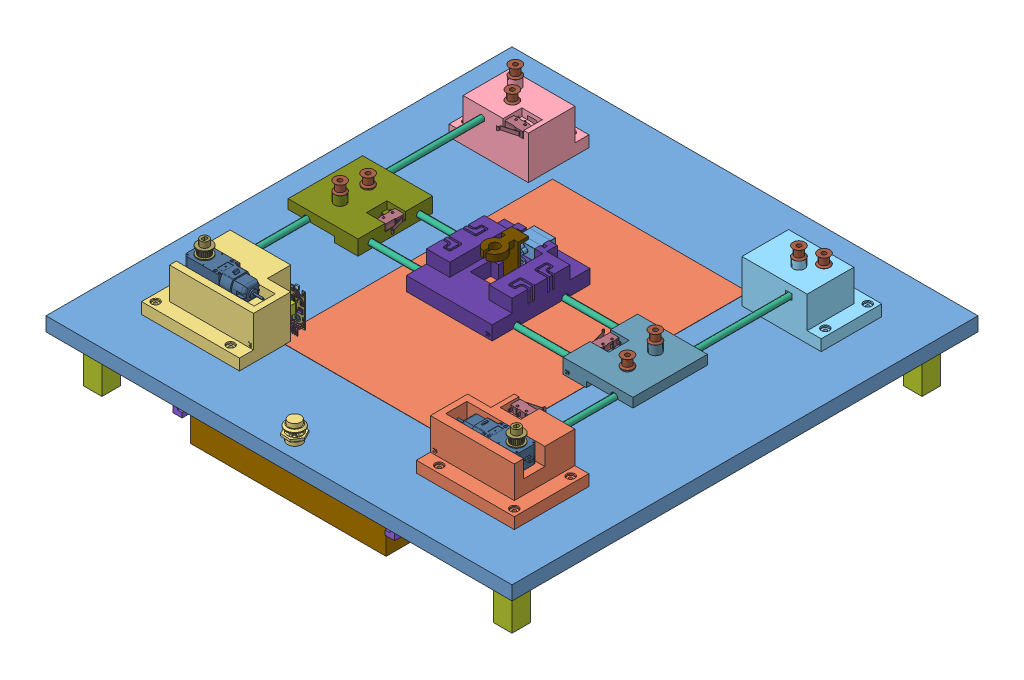
SolidWorks assembly Assem1.1, configuration Default. Lengths in mm.
Overall size (500 139.59 500).
80 component instances, 49 part files, 171 mates.
Components (placement in the parent):
- Base-1: Base [Default] at (441.6833 230.1614 146.9363) size (500 15 500)
- STEPPER RIGHT-1: STEPPER RIGHT [Default] at (291.6086 245.1614 514.4363) size (105 46 80)
- STEPPER LEFT-1: STEPPER LEFT [Default] at (91.7583 245.1614 579.4363) x (0 0 1) z (0 1 0) size (80 105 46)
- TOP RIGHT-1: TOP RIGHT [Default] at (6.7583 245.1614 214.4363) size (85 56 65)
- TOP LEFT-1: TOP LEFT [Default] at (377.872 245.1614 264.4363) x (0 0 1) z (-1 0 0) size (65 54.7 85)
- Shaft-2: Shaft [Default] at (26.7583 280.1614 234.4363) x (0.670425 0.741977 0) z (0.741977 -0.670425 0) size (6 300 6)
- FOOT-1: FOOT [Default] at (-38.3167 180.1614 606.9363) size (40 50 40)
- FOOT-2: FOOT [Default] at (401.6833 180.1614 606.9363) size (40 50 40)
- FOOT-3: FOOT [Default] at (401.6833 180.1614 166.9363) size (40 50 40)
- FOOT-4: FOOT [Default] at (-38.3167 180.1614 166.9363) size (40 50 40)
- STORAGE SUPPORT-1: STORAGE SUPPORT [Default] at (318.6833 225.1614 481.9363) x (-1 0 0) z (0 1 0) size (18 160 12)
- STORAGE SUPPORT-2: STORAGE SUPPORT [Default] at (64.6833 225.1614 641.9363) x (1 0 0) z (0 1 0) size (18 160 12)
- STORAGE-2: STORAGE [Default] at (91.6833 199.1614 632.0504) x (1 0 0) z (0 0 -1) size (226 35 155)
- DG01D Motor-1: DG01D Motor [Default] at (25.7583 300.9614 560.8363) x (-1 0 0) z (0 1 0) size (79.2 22.5 37.6)
- DG01D Motor-2: DG01D Motor [Default] at (357.6086 291.1614 558.0363) x (1 0 0) z (0 1 0) size (79.2 22.5 37.6)
- Pully-3: Pully [Default] at (345.0586 304.8614 242.4363) x (-1 0 0) z (0 0 1) size (12.7 10 12.7)
- Pully-4: Pully [Default] at (356.9086 296.1614 227.4363) x (-1 0 0) z (0 0 1) size (12.7 10 12.7)
- GT2 20T motor-1: GT2 20T motor [Default] at (25.7583 309.4614 560.8363) x (1 0 0) z (0 1 0) size (16 16 15)
- GT2 20T motor-2: GT2 20T motor [Default] at (357.6086 299.6614 558.0363) x (1 0 0) z (0 1 0) size (16 16 15)
- Pully-9: Pully [Default] at (25.7583 306.1614 227.4363) x (-1 0 0) z (0 0 1) size (12.7 10 12.7)
- Pully-10: Pully [Default] at (37.6083 296.1614 242.4363) x (-1 0 0) z (0 0 1) size (12.7 10 12.7)
- SS_5GL13.step-3: SS_5GL13.step [Default] at (332.3586 286.3614 522.1363) x (1 0 0) z (0 1 0) size (21.03 22.89 6.4)
- SS_5GL13.step-4: SS_5GL13.step [Default] at (56.0083 286.3614 256.7363) x (-1 0 0) z (0 1 0) size (21.03 22.89 6.4)
- Shaft-8: Shaft [Default] at (356.7586 280.0114 234.4363) x (-0.419242 0.907875 0) z (0.907875 0.419242 0) size (6 300 6)
- END EFFECTOR RIGHT-3: END EFFECTOR RIGHT [Default] at (316.7592 279.469 452.2484) x (0 0 -1) z (0.999999 0.001061 0) size (80 26 75)
- LMU-N6-8: LMU-N6 [Default] at (356.7586 280.0114 411.9984) x (-0.078757 0.996894 0) z (0.996894 0.078757 0) size (12 19 12)
- LMU-N6-9: LMU-N6 [Default] at (26.7583 280.1614 411.9984) x (1 0 0) z (0 1 0) size (12 19 12)
- END EFFECTOR LEFT-3: END EFFECTOR LEFT [Default] at (66.7593 279.2038 372.2484) x (0 0 1) z (-0.999999 -0.001061 0) size (80 26 75)
- Shaft-9: Shaft [Default] at (341.7591 279.4955 438.2484) x (-0.000465 0.43872 0.898624) z (0.000953 -0.898623 0.43872) size (6 300 6)
- Shaft-10: Shaft [Default] at (341.7591 279.4955 386.2484) x (-0.001061 0.999999 0) z (0 0 1) size (6 300 6)
- END EFFECTOR BASE-3: END EFFECTOR BASE [Default] at (238.2479 278.8857 464.7484) x (0 0 -1) z (0.999999 0.001061 0) size (105 29 92)
- LMU-N6-10: LMU-N6 [Default] at (168.7474 279.312 386.2484) x (0.001061 -0.999999 0) z (0 0 1) size (12 19 12)
- LMU-N6-11: LMU-N6 [Default] at (191.7474 279.3364 438.2484) x (0.001043 -0.983378 -0.181565) z (0.000193 -0.181565 0.983379) size (12 19 12)
- LMU-N6-12: LMU-N6 [Default] at (215.7474 279.3618 386.2484) x (0.001061 -0.999999 0) z (0 0 1) size (12 19 12)
- PEN HOLDER NEW-2: PEN HOLDER NEW [Default] at (192.212 312.7416 415.8858) x (0.999999 0.001061 0) z (0 0 1) size (22 52.5 38.03)
- SS_5GL13.step-5: SS_5GL13.step [Default] at (309.4536 284.6612 407.4984) x (0 0 -1) z (-0.001061 0.999999 0) size (21.03 22.89 6.4)
- SS_5GL13.step-6: SS_5GL13.step [Default] at (74.0538 284.4116 416.9984) x (0 0 1) z (-0.001061 0.999999 0) size (21.03 22.89 6.4)
- Pully-11: Pully [Default] at (345.8915 296.0999 427.2484) x (-0.999999 -0.001061 0) z (0 0 1) size (12.7 10 12.7)
- Pully-12: Pully [Default] at (345.8826 304.4999 397.2484) x (-0.999999 -0.001061 0) z (0 0 1) size (12.7 10 12.7)
- Pully-13: Pully [Default] at (37.5828 304.1729 427.2484) x (0.837232 0.000888 0.546848) z (0.546847 0.00058 -0.837232) size (12.7 10 12.7)
- Pully-14: Pully [Default] at (37.5917 295.7729 397.2484) x (-0.999999 -0.001061 0) z (0 0 1) size (12.7 10 12.7)
- servo-1: servo [Default] at (184.3266 318.5665 361.0815) x (0.999999 0.001061 0) z (0.001061 -0.999999 0) size (38.73 33.09 12.1)
- A4_paper-1: A4_paper [Default] at (191.6833 245.1614 396.9363) size (210 0.3 297)
- PushButtonRed-1: PushButtonRed [Default] at (191.0864 258.4614 629.4531) x (-0.837169 0 -0.546944) z (0 1 0) size (19.62 21.94 25.6)
- KY-024 Linear Magnetic Hall Effect Switches.step-3: KY-024 Linear Magnetic Hall Effect Switches.step [Default] at (93.976 267.3857 527.7213) x (0 1 0) z (1 0 0) size (43.63 13.45 15)
  - Sensor.step-1: Sensor.step [Default] at (21.0875 1.0886 -0.8799) x (0 0 -1) z (0 -1 0) size (6.43 12.72 3.32)
    - Pins.step-1: Pins.step [Default] at origin size (5.99 9.68 3.16)
    - Sensor-0.step-1: Sensor-0.step [Default] at origin size (4.1 3.2 1.5)
  - Fusion002.step-1: Fusion002.step [Default] at (2.0698 -0.285 -0.8494) x (0 0 1) z (0 1 0) size (14.06 29.56 0.01)
  - Trimpot.step-1: Trimpot.step [Default] at (0.8941 5.715 -1.9169) x (0 1 0) z (1 0 0) size (13.19 5 10)
  - lm393.step-1: lm393.step [Default] at (16.3888 -1.3356 -7.4144) x (-1 0 0) z (0 1 0) size (4.98 4.98 1.83)
  - Pad003.step-1: Pad003.step [Default] at (2.0698 0.725 -0.8494) x (0 0 1) z (0 1 0) size (14.68 24.36 0.01)
  - Pad001.step-1: Pad001.step [Default] at (2.0698 -0.294 -0.8494) x (0 0 1) z (0 1 0) size (13.63 28.59 1.03)
  - Pad002.step-1: Pad002.step [Default] at (2.0698 0.725 -0.8494) x (0 0 1) z (0 1 0) size (9.53 3.34 0.01)
  - PCB.step-1: PCB.step [Default] at (2.0698 -0.285 -0.8494) x (0 0 1) z (0 1 0) size (15 35 1)
  - PIN HEADER, 1X4, 2.54 mm.step-1: PIN HEADER, 1X4, 2.54 mm.step [Default] at (-13.6966 0.693 -2.0725) x (0 0 -1) z (1 0 0) size (10.08 6.81 8.5)
  - Led.step-1: Led.step [Default] at (0.9398 -1.2392 1.8074) x (-1 0 0) z (0 1 0) size (2.66 1.33 0.62)
  - Led (1).step-1: Led (1).step [Default] at (2.913 -0.8113 -18.8497) size (2.66 0.62 1.33)
  - Resistor.step-1: Resistor.step [Default] at origin size (2.57 0.86 1.53)
  - Resistor (1).step-1: Resistor (1).step [Default] at (0 0 -2.456) size (2.57 0.86 1.53)
  - Resistor (2).step-1: Resistor (2).step [Default] at (0 0 -9.9569) size (2.57 0.86 1.53)
  - Resistor (3).step-1: Resistor (3).step [Default] at (0 0 -12.4652) size (2.57 0.86 1.53)
  - Resistor (4).step-1: Resistor (4).step [Default] at (-18.4143 0 0.076) size (2.57 0.86 1.53)
  - Resistor (5).step-1: Resistor (5).step [Default] at (-18.5044 0 -12.6045) size (2.57 0.86 1.53)
  - Pad (2).step-1: Pad (2).step [Default] at origin size (1.8 0.7 1.8)
  - Pad (4).step-1: Pad (4).step [Default] at origin size (1.8 0.7 1.8)
  - Pad (3).step-1: Pad (3).step [Default] at origin size (1.8 0.7 1.8)
  - Pad (5).step-1: Pad (5).step [Default] at origin size (1.8 0.7 1.8)
  - Pad (2) (1).step-1: Pad (2) (1).step [Default] at (12.1225 0 -7.5843) size (1.8 0.7 1.8)
  - Pad (2) (2).step-1: Pad (2) (2).step [Default] at (14.6713 0 -7.6465) size (1.8 0.7 1.8)
  - Pad (2) (3).step-1: Pad (2) (3).step [Default] at (17.0958 0 -7.5843) size (1.8 0.7 1.8)
  - Pad.step-1: Pad.step [Default] at origin size (1.6 1.01 1.6)
  - Pad (1).step-1: Pad (1).step [Default] at origin size (1.6 1.01 1.6)
  - Pad (6).step-1: Pad (6).step [Default] at origin size (1.6 1.01 1.6)
  - Pad (2) (3).step-2: Pad (2) (3).step [Default] at (23.9554 0.5875 6.0878) x (1 0 0) z (0 0 -1) size (1.8 0.7 1.8)
  - Pad (2) (3).step-3: Pad (2) (3).step [Default] at (25.2062 0.5875 3.4651) x (1 0 0) z (0 0 -1) size (1.8 0.7 1.8)
  - Pad (2) (3).step-4: Pad (2) (3).step [Default] at (25.2466 0.5875 0.8827) x (1 0 0) z (0 0 -1) size (1.8 0.7 1.8)
  - Pad (2) (3).step-5: Pad (2) (3).step [Default] at (25.2466 -0.0666 -4.9814) size (1.8 0.7 1.8)
  - Pad (2) (3).step-6: Pad (2) (3).step [Default] at (25.2466 -0.0666 -2.5658) size (1.8 0.7 1.8)
  - Pad (2) (3).step-7: Pad (2) (3).step [Default] at (23.8777 -0.0666 0.2122) size (1.8 0.7 1.8)
Mates (geometry in assembly coordinates):
- Coincident1: coincident anti-aligned: plane of Base-1 through (441.6833 245.1614 146.9363) normal (0 1 0); plane of STEPPER RIGHT-1 through (291.6086 245.1614 514.4363) normal (0 -1 0)
- Coincident2: coincident anti-aligned: plane of Base-1 through (441.6833 245.1614 146.9363) normal (0 1 0); plane of STEPPER LEFT-1 through (91.7583 245.1614 579.4363) normal (0 -1 0)
- Coincident3: coincident anti-aligned: plane of Base-1 through (441.6833 245.1614 146.9363) normal (0 1 0); plane of TOP RIGHT-1 through (6.7583 245.1614 214.4363) normal (0 -1 0)
- Coincident4: coincident anti-aligned: plane of Base-1 through (441.6833 245.1614 146.9363) normal (0 1 0); plane of TOP LEFT-1 through (377.872 245.1614 264.4363) normal (0 -1 0)
- Tangent12: tangent anti-aligned: plane of TOP LEFT-1 through (352.7586 277.0114 234.4363) normal (0 1 0); cylinder of Shaft-3 through (357.1083 280.0114 529.4363) axis (0 0 -1) radius 3
- Concentric3: concentric anti-aligned: cylinder of Shaft-3 through (357.1083 280.0114 529.4363) axis (0 0 -1) radius 3; cylinder of LMU-N6-1 through (376.7583 280.0114 378.9727) axis (0 0 1) radius 3
- Concentric4: concentric aligned: cylinder of END EFFECTOR LEFT-1 through (376.7583 280.0114 378.4727) axis (0 0 1) radius 6; cylinder of LMU-N6-1 through (376.7583 280.0114 378.9727) axis (0 0 1) radius 6
- Coincident13: coincident anti-aligned: plane of END EFFECTOR LEFT-1 through (376.7583 280.0114 397.9727) normal (0 0 -1); plane of LMU-N6-1 through (376.7583 280.0114 397.9727) normal (0 0 1)
- Concentric5: concentric aligned: cylinder of Shaft-2 through (26.7583 280.1614 534.4363) axis (0 0 -1) radius 3; cylinder of LMU-N6-2 through (46.7579 280.1614 397.4727) axis (0 0 -1) radius 3
- Concentric6: concentric aligned: cylinder of END EFFECTOR RIGHT-1 through (46.7579 280.1614 397.9727) axis (0 0 -1) radius 6; cylinder of LMU-N6-2 through (46.7579 280.1614 397.4727) axis (0 0 -1) radius 6
- Coincident14: coincident anti-aligned: plane of END EFFECTOR RIGHT-1 through (46.7579 280.1614 378.4727) normal (0 0 1); plane of LMU-N6-2 through (46.7579 280.1614 378.4727) normal (0 0 -1)
- Concentric7: concentric anti-aligned: cylinder of END EFFECTOR LEFT-1 through (361.7563 279.0409 414.2227) axis (-0.999998 0.00197 0) radius 3.15; cylinder of Shaft-4 through (61.7569 279.6319 414.2227) axis (0.999998 -0.00197 0) radius 3
- Coincident15: coincident anti-aligned: plane of END EFFECTOR LEFT-1 through (361.7563 279.0409 414.2227) normal (-0.999998 0.00197 0); plane of Shaft-4 through (361.7563 279.0409 414.2227) normal (0.999998 -0.00197 0)
- Concentric8: concentric anti-aligned: cylinder of END EFFECTOR LEFT-1 through (361.7563 279.0409 362.2227) axis (-0.999998 0.00197 0) radius 3.15; cylinder of Shaft-5 through (61.7569 279.6319 362.2227) axis (0.999998 -0.00197 0) radius 3
- Coincident16: coincident anti-aligned: plane of END EFFECTOR LEFT-1 through (361.7563 279.0409 362.2227) normal (-0.999998 0.00197 0); plane of Shaft-5 through (361.7563 279.0409 362.2227) normal (0.999998 -0.00197 0)
- Coincident17: coincident anti-aligned: plane of END EFFECTOR RIGHT-1 through (61.7569 279.6319 414.2227) normal (0.999998 -0.00197 0); plane of Shaft-4 through (61.7569 279.6319 414.2227) normal (-0.999998 0.00197 0)
- Coincident18: coincident anti-aligned: plane of END EFFECTOR RIGHT-1 through (61.7569 279.6319 362.2227) normal (0.999998 -0.00197 0); plane of Shaft-5 through (61.7569 279.6319 362.2227) normal (-0.999998 0.00197 0)
- Concentric9: concentric aligned: cylinder of END EFFECTOR RIGHT-1 through (61.7569 279.6319 362.2227) axis (0.999998 -0.00197 0) radius 3.15; cylinder of Shaft-5 through (61.7569 279.6319 362.2227) axis (0.999998 -0.00197 0) radius 3
- Concentric10: concentric anti-aligned: cylinder of Shaft-5 through (61.7569 279.6319 362.2227) axis (0.999998 -0.00197 0) radius 3; cylinder of LMU-N6-3 through (251.3995 279.2583 362.2227) axis (-0.999998 0.00197 0) radius 3
- Concentric11: concentric aligned: cylinder of Shaft-5 through (61.7569 279.6319 362.2227) axis (0.999998 -0.00197 0) radius 3; cylinder of LMU-N6-4 through (187.3997 279.3844 362.2227) axis (0.999998 -0.00197 0) radius 3
- Concentric12: concentric anti-aligned: cylinder of Shaft-4 through (61.7569 279.6319 414.2227) axis (0.999998 -0.00197 0) radius 3; circle of LMU-N6-5
- Concentric13: concentric aligned: cylinder of END EFFECTOR BASE-2 through (229.3996 279.3017 414.2227) axis (-0.999998 0.00197 0) radius 6; cylinder of LMU-N6-5 through (228.3996 279.3036 414.2227) axis (-0.999998 0.00197 0) radius 6
- Coincident19: coincident anti-aligned: plane of END EFFECTOR BASE-2 through (209.3996 279.341 414.2227) normal (0.999998 -0.00197 0); plane of LMU-N6-5 through (209.3996 279.341 414.2227) normal (-0.999998 0.00197 0)
- Concentric14: concentric aligned: cylinder of END EFFECTOR BASE-2 through (252.3995 279.2563 362.2227) axis (-0.999998 0.00197 0) radius 6; cylinder of LMU-N6-3 through (251.3995 279.2583 362.2227) axis (-0.999998 0.00197 0) radius 6
- Concentric15: concentric aligned: cylinder of END EFFECTOR BASE-2 through (186.3997 279.3863 362.2227) axis (0.999998 -0.00197 0) radius 6; cylinder of LMU-N6-4 through (187.3997 279.3844 362.2227) axis (0.999998 -0.00197 0) radius 6
- Coincident20: coincident anti-aligned: plane of END EFFECTOR BASE-2 through (206.3996 279.347 362.2227) normal (-0.999998 0.00197 0); plane of LMU-N6-4 through (206.3996 279.347 362.2227) normal (0.999998 -0.00197 0)
- Coincident21: coincident anti-aligned: plane of END EFFECTOR BASE-2 through (232.3996 279.2957 362.2227) normal (0.999998 -0.00197 0); plane of LMU-N6-3 through (232.3996 279.2957 362.2227) normal (-0.999998 0.00197 0)
- Coincident22: coincident: plane of END EFFECTOR BASE-2 through (265.4281 293.7307 440.7227) normal (0.00197 0.999998 0); plane of END EFFECTOR TOP-1 through (212.6755 294.0223 310.2117) normal (-0.000676 -1 0)
- Coincident23: coincident anti-aligned: plane of END EFFECTOR BASE-2 through (234.2863 221.7919 373.2227) normal (0 0 1); plane of PEN HOLDER NEW-1 through (219.4672 313.617 373.2227) normal (0 0 -1)
- Distance7: distance = 1 mm anti-aligned: plane of PEN HOLDER NEW-1 through (228.4671 313.5993 373.2227) normal (0.999998 -0.00197 0); plane of END EFFECTOR BASE-2 through (229.3986 278.8017 373.2227) normal (-0.999998 0.00197 0)
- Coincident26: coincident anti-aligned: plane of Base-1 through (441.6833 230.1614 146.9363) normal (0 -1 0); plane of FOOT-1 through (-38.3167 230.1614 606.9363) normal (0 1 0)
- Distance10: distance = 10 mm aligned: plane of Base-1 through (-58.3167 245.1614 146.9363) normal (-1 0 0); plane of FOOT-1 through (-48.3167 225.1614 596.9363) normal (-1 0 0)
- Distance11: distance = 10 mm aligned: plane of FOOT-1 through (-48.3167 225.1614 636.9363) normal (0 0 1); plane of Base-1 through (441.6833 245.1614 646.9363) normal (0 0 1)
- Coincident28: coincident anti-aligned: plane of Base-1 through (441.6833 230.1614 146.9363) normal (0 -1 0); plane of FOOT-2 through (401.6833 230.1614 606.9363) normal (0 1 0)
- Distance13: distance = 10 mm aligned: plane of FOOT-2 through (391.6833 225.1614 636.9363) normal (0 0 1); plane of Base-1 through (441.6833 245.1614 646.9363) normal (0 0 1)
- Distance14: distance = 10 mm aligned: plane of FOOT-2 through (431.6833 225.1614 596.9363) normal (1 0 0); plane of Base-1 through (441.6833 245.1614 146.9363) normal (1 0 0)
- Coincident31: coincident anti-aligned: plane of Base-1 through (441.6833 230.1614 146.9363) normal (0 -1 0); plane of FOOT-3 through (401.6833 230.1614 166.9363) normal (0 1 0)
- Distance15: distance = 10 mm aligned: plane of FOOT-3 through (431.6833 225.1614 156.9363) normal (1 0 0); plane of Base-1 through (441.6833 245.1614 146.9363) normal (1 0 0)
- Distance16: distance = 10 mm aligned: plane of FOOT-3 through (391.6833 225.1614 156.9363) normal (0 0 -1); plane of Base-1 through (441.6833 245.1614 146.9363) normal (0 0 -1)
- Coincident34: coincident anti-aligned: plane of Base-1 through (441.6833 230.1614 146.9363) normal (0 -1 0); plane of FOOT-4 through (-38.3167 230.1614 166.9363) normal (0 1 0)
- Distance17: distance = 10 mm aligned: plane of FOOT-4 through (-48.3167 225.1614 156.9363) normal (0 0 -1); plane of Base-1 through (441.6833 245.1614 146.9363) normal (0 0 -1)
- Distance18: distance = 10 mm aligned: plane of FOOT-4 through (-48.3167 225.1614 156.9363) normal (-1 0 0); plane of Base-1 through (-58.3167 245.1614 146.9363) normal (-1 0 0)
- Coincident37: coincident anti-aligned: plane of Base-1 through (441.6833 230.1614 146.9363) normal (0 -1 0); plane of STORAGE SUPPORT-1 through (310.6833 230.1614 641.9363) normal (0 1 0)
- Coincident38: coincident anti-aligned: plane of Base-1 through (441.6833 230.1614 146.9363) normal (0 -1 0); plane of STORAGE SUPPORT-2 through (72.6833 230.1614 481.9363) normal (0 1 0)
- Distance19: distance = 1 mm anti-aligned: plane of STORAGE-2 through (91.6833 229.1614 632.0504) normal (0 1 0); plane of Base-1 through (441.6833 230.1614 146.9363) normal (0 -1 0)
- Distance20: distance = 137 mm aligned: plane of STORAGE-2 through (304.6833 199.1614 632.0504) normal (1 0 0); plane of Base-1 through (441.6833 245.1614 146.9363) normal (1 0 0)
- Distance22: distance = 1 mm anti-aligned: plane of STORAGE-2 through (304.6833 199.1614 632.0504) normal (1 0 0); plane of STORAGE SUPPORT-1 through (305.6833 230.1614 641.9363) normal (-1 0 0)
- Distance23: distance = 1 mm anti-aligned: plane of STORAGE SUPPORT-2 through (77.6833 230.1614 481.9363) normal (1 0 0); plane of STORAGE-2 through (78.6833 199.1614 632.0504) normal (-1 0 0)
- Distance24: distance = 5 mm aligned: plane of STORAGE SUPPORT-1 through (318.6833 225.1614 641.9363) normal (0 0 1); plane of Base-1 through (441.6833 245.1614 646.9363) normal (0 0 1)
- Distance25: distance = 5 mm aligned: plane of STORAGE SUPPORT-2 through (64.6833 225.1614 641.9363) normal (0 0 1); plane of Base-1 through (441.6833 245.1614 646.9363) normal (0 0 1)
- Concentric16: concentric anti-aligned: cylinder of STEPPER LEFT-1 through (25.7583 228.7114 560.8363) axis (0 1 0) radius 3.25; cylinder of DG01D Motor-1 through (25.7583 291.5645 560.8363) axis (0 -1 0) radius 2.6
- Concentric17: concentric aligned: cylinder of STEPPER LEFT-1 through (38.0583 228.7114 560.8363) axis (0 1 0) radius 2.35; cylinder of DG01D Motor-1 through (38.0583 281.4193 560.8363) axis (0 1 0) radius 1.9
- Coincident39: coincident anti-aligned: plane of STEPPER LEFT-1 through (91.7583 282.1614 579.4363) normal (0 1 0); plane of DG01D Motor-1 through (32.8456 282.1614 559.8363) normal (0 -1 0)
- Concentric18: concentric anti-aligned: cylinder of STEPPER RIGHT-1 through (357.6086 245.3614 558.0363) axis (0 1 0) radius 3.25; cylinder of DG01D Motor-2 through (357.6086 281.7645 558.0363) axis (0 -1 0) radius 2.6
- Concentric19: concentric aligned: cylinder of STEPPER RIGHT-1 through (345.3086 245.3614 558.0363) axis (0 1 0) radius 2.35; cylinder of DG01D Motor-2 through (345.3086 271.6193 558.0363) axis (0 1 0) radius 1.9
- Coincident40: coincident anti-aligned: plane of STEPPER RIGHT-1 through (291.6086 272.3614 514.4363) normal (0 1 0); plane of DG01D Motor-2 through (350.5212 272.3614 559.0363) normal (0 -1 0)
- Coincident43: coincident anti-aligned: plane of TOP LEFT-1 through (345.0586 299.8614 242.4363) normal (0 1 0); plane of Pully-3 through (345.0586 299.8614 236.0863) normal (0 -1 0)
- Concentric22: concentric aligned: circle of TOP LEFT-1; cylinder of Pully-3 through (345.0586 304.8614 242.4363) axis (0 1 0) radius 2.35
- Coincident44: coincident anti-aligned: plane of TOP LEFT-1 through (377.872 291.1614 264.4363) normal (0 1 0); plane of Pully-4 through (356.9086 291.1614 221.0863) normal (0 -1 0)
- Concentric23: concentric aligned: cylinder of TOP LEFT-1 through (356.9086 281.1614 227.4363) axis (0 1 0) radius 2.5; circle of Pully-4
- Coincident45: coincident anti-aligned: plane of END EFFECTOR LEFT-1 through (365.9457 299.0327 373.2227) normal (0.00197 0.999998 0); plane of Pully-5 through (365.9457 299.0327 366.8727) normal (-0.00197 -0.999998 0)
- Concentric24: concentric aligned: cylinder of END EFFECTOR LEFT-1 through (365.8866 269.0328 373.2227) axis (0.00197 0.999998 0) radius 2.5; cylinder of Pully-5 through (365.9556 304.0327 373.2227) axis (0.00197 0.999998 0) radius 2.35
- Coincident46: coincident anti-aligned: plane of END EFFECTOR LEFT-1 through (365.9292 290.6328 403.2227) normal (0.00197 0.999998 0); plane of Pully-6 through (365.9292 290.6328 396.8727) normal (-0.00197 -0.999998 0)
- Concentric25: concentric aligned: cylinder of END EFFECTOR LEFT-1 through (365.8866 269.0328 403.2227) axis (0.00197 0.999998 0) radius 2.5; cylinder of Pully-6 through (365.939 295.6327 403.2227) axis (0.00197 0.999998 0) radius 2.35
- Coincident49: coincident anti-aligned: plane of DG01D Motor-2 through (350.5212 291.1614 557.0363) normal (0 1 0); plane of gear_pulley_V2.stp-1 through (377.6083 291.1614 563.0363) normal (0 -1 0)
- Concentric28: concentric anti-aligned: cylinder of DG01D Motor-2 through (357.6086 262.9645 558.0363) axis (0 -1 0) radius 1.2093; cylinder of gear_pulley_V2.stp-1 through (377.6083 314.6614 563.0363) axis (0 1 0) radius 1.8
- Coincident50: coincident: plane of DG01D Motor-1 through (32.8456 300.9614 561.8363) normal (0 1 0); plane of gear_pulley_V2.stp-3 through (5.7583 300.9614 565.8363) normal (0 -1 0)
- Concentric29: concentric: cylinder of DG01D Motor-1 through (25.7583 272.7645 560.8363) axis (0 -1 0) radius 1.2093; cylinder of gear_pulley_V2.stp-3 through (5.7583 324.4614 565.8363) axis (0 1 0) radius 1.8
- Coincident51: coincident anti-aligned: plane of DG01D Motor-1 through (32.8456 300.9614 561.8363) normal (0 1 0); plane of GT2 20T motor-1 through (25.7583 300.9614 560.8363) normal (0 -1 0)
- Concentric30: concentric anti-aligned: cylinder of DG01D Motor-1 through (25.7583 272.7645 560.8363) axis (0 -1 0) radius 1.2093; cylinder of GT2 20T motor-1 through (25.7583 309.4614 560.8363) axis (0 1 0) radius 2.6
- Coincident52: coincident anti-aligned: plane of DG01D Motor-2 through (350.5212 291.1614 557.0363) normal (0 1 0); plane of GT2 20T motor-2 through (357.6086 291.1614 558.0363) normal (0 -1 0)
- Concentric31: concentric anti-aligned: cylinder of DG01D Motor-2 through (357.6086 281.7645 558.0363) axis (0 -1 0) radius 2.6; cylinder of GT2 20T motor-2 through (357.6086 299.6614 558.0363) axis (0 1 0) radius 2.6
- Coincident53: coincident anti-aligned: plane of END EFFECTOR RIGHT-1 through (57.6463 299.64 403.2227) normal (0.00197 0.999998 0); plane of Pully-7 through (57.6463 299.64 396.8727) normal (-0.00197 -0.999998 0)
- Concentric32: concentric aligned: circle of END EFFECTOR RIGHT-1; circle of Pully-7
- Coincident54: coincident anti-aligned: plane of END EFFECTOR RIGHT-1 through (57.6298 291.24 373.2227) normal (0.00197 0.999998 0); plane of Pully-8 through (57.6298 291.24 366.8727) normal (-0.00197 -0.999998 0)
- Concentric33: concentric aligned: circle of END EFFECTOR RIGHT-1; circle of Pully-8
- Coincident55: coincident anti-aligned: plane of TOP RIGHT-1 through (25.7583 301.1614 227.4363) normal (0 1 0); plane of Pully-9 through (25.7583 301.1614 221.0863) normal (0 -1 0)
- Concentric34: concentric aligned: cylinder of TOP RIGHT-1 through (25.7583 281.1614 227.4363) axis (0 1 0) radius 2.5; circle of Pully-9
- Coincident56: coincident anti-aligned: plane of TOP RIGHT-1 through (6.7583 291.1614 214.4363) normal (0 1 0); plane of Pully-10 through (37.6083 291.1614 236.0863) normal (0 -1 0)
- Concentric35: concentric aligned: cylinder of TOP RIGHT-1 through (37.6083 281.1614 242.4363) axis (0 1 0) radius 2.5; cylinder of Pully-10 through (37.6083 296.1614 242.4363) axis (0 1 0) radius 2.35
- Concentric36: concentric aligned: cylinder of END EFFECTOR RIGHT-1 through (94.0214 261.5683 392.9727) axis (0.00197 0.999998 0) radius 1.185; cylinder of SS_5GL13.step-1 through (94.0608 281.5682 392.9727) axis (0.00197 0.999998 0) radius 1.175
- Concentric37: concentric aligned: cylinder of END EFFECTOR RIGHT-1 through (94.0214 261.5683 383.4727) axis (0.00197 0.999998 0) radius 1.185; cylinder of SS_5GL13.step-1 through (94.0608 281.5682 383.4727) axis (0.00197 0.999998 0) radius 1.25
- Parallel1: parallel aligned: plane of END EFFECTOR RIGHT-1 through (101.7568 279.5531 414.2227) normal (0.999998 -0.00197 0); plane of SS_5GL13.step-1 through (101.0734 287.9544 388.0727) normal (0.999998 -0.00197 0)
- Coincident57: coincident anti-aligned: plane of END EFFECTOR RIGHT-1 through (81.7608 281.5925 399.2227) normal (0.00197 0.999998 0); plane of SS_5GL13.step-1 through (91.5608 281.5732 398.1727) normal (-0.00197 -0.999998 0)
- Concentric38: concentric aligned: cylinder of END EFFECTOR LEFT-1 through (329.4209 261.1046 383.4727) axis (0.00197 0.999998 0) radius 1.185; cylinder of SS_5GL13.step-2 through (329.4603 281.1046 383.4727) axis (0.00197 0.999998 0) radius 1.175
- Parallel2: parallel aligned: plane of END EFFECTOR LEFT-1 through (321.7564 279.1197 362.2227) normal (-0.999998 0.00197 0); plane of SS_5GL13.step-2 through (322.4729 287.5183 388.3727) normal (-0.999998 0.00197 0)
- Coincident58: coincident anti-aligned: plane of END EFFECTOR LEFT-1 through (341.7603 281.0803 377.2227) normal (0.00197 0.999998 0); plane of SS_5GL13.step-2 through (331.9603 281.0996 378.2727) normal (-0.00197 -0.999998 0)
- Coincident59: coincident anti-aligned: plane of STEPPER RIGHT-1 through (338.6086 283.1614 534.4363) normal (0 1 0); plane of SS_5GL13.step-3 through (337.5586 283.1614 524.6363) normal (0 -1 0)
- Concentric40: concentric aligned: cylinder of STEPPER RIGHT-1 through (332.3586 273.1614 522.1363) axis (0 1 0) radius 1.185; cylinder of SS_5GL13.step-3 through (332.3586 283.1614 522.1363) axis (0 1 0) radius 1.175
- Concentric41: concentric aligned: cylinder of STEPPER RIGHT-1 through (322.8586 273.1614 522.1363) axis (0 1 0) radius 1.185; cylinder of SS_5GL13.step-3 through (322.8586 283.1614 522.1363) axis (0 1 0) radius 1.25
- Concentric42: concentric aligned: cylinder of TOP RIGHT-1 through (65.5083 273.1614 256.7363) axis (0 1 0) radius 1.185; cylinder of SS_5GL13.step-4 through (65.5083 283.1614 256.7363) axis (0 1 0) radius 1.25
- Concentric43: concentric aligned: circle of TOP RIGHT-1; cylinder of SS_5GL13.step-4 through (56.0083 283.1614 256.7363) axis (0 1 0) radius 1.175
- Coincident60: coincident anti-aligned: plane of TOP RIGHT-1 through (49.7583 283.1614 244.4363) normal (0 1 0); plane of SS_5GL13.step-4 through (50.8083 283.1614 254.2363) normal (0 -1 0)
- Concentric44: concentric aligned: cylinder of Shaft-3 through (357.1083 280.0114 529.4363) axis (0 0 -1) radius 3; cylinder of LMU-N6-6 through (357.1083 280.0114 403.3764) axis (0 0 -1) radius 3
- Concentric45: concentric anti-aligned: cylinder of END EFFECTOR RIGHT-2 through (357.1083 280.0114 383.8764) axis (0 0 1) radius 6; cylinder of LMU-N6-6 through (357.1083 280.0114 403.3764) axis (0 0 -1) radius 6
- Coincident61: coincident anti-aligned: plane of END EFFECTOR RIGHT-2 through (357.1083 280.0114 403.3764) normal (0 0 -1); plane of LMU-N6-6 through (357.1083 280.0114 403.3764) normal (0 0 1)
- Concentric46: concentric anti-aligned: cylinder of Shaft-2 through (26.7583 280.1614 534.4363) axis (0 0 -1) radius 3; cylinder of LMU-N6-7 through (27.1079 280.1614 383.8764) axis (0 0 1) radius 3
- Concentric47: concentric anti-aligned: cylinder of END EFFECTOR LEFT-2 through (27.1079 280.1614 403.3764) axis (0 0 -1) radius 6; cylinder of LMU-N6-7 through (27.1079 280.1614 383.8764) axis (0 0 1) radius 6
- Coincident62: coincident anti-aligned: plane of END EFFECTOR LEFT-2 through (27.1079 280.1614 383.8764) normal (0 0 1); plane of LMU-N6-7 through (27.1079 280.1614 383.8764) normal (0 0 -1)
- Concentric48: concentric aligned: cylinder of END EFFECTOR RIGHT-2 through (342.1088 279.4955 367.6264) axis (-0.999999 -0.001061 0) radius 3.15; cylinder of Shaft-6 through (342.1088 279.4955 367.6264) axis (-0.999999 -0.001061 0) radius 3
- Coincident63: coincident anti-aligned: plane of END EFFECTOR RIGHT-2 through (342.1088 279.4955 367.6264) normal (-0.999999 -0.001061 0); plane of Shaft-6 through (342.1088 279.4955 367.6264) normal (0.999999 0.001061 0)
- Concentric49: concentric anti-aligned: cylinder of END EFFECTOR LEFT-2 through (42.109 279.1773 367.6264) axis (0.999999 0.001061 0) radius 3.15; cylinder of Shaft-6 through (342.1088 279.4955 367.6264) axis (-0.999999 -0.001061 0) radius 3
- Coincident64: coincident aligned: plane of END EFFECTOR LEFT-2 through (42.109 279.1773 367.6264) normal (0.999999 0.001061 0); circle of Shaft-6
- Concentric50: concentric anti-aligned: cylinder of END EFFECTOR RIGHT-2 through (342.1088 279.4955 419.6264) axis (-0.999999 -0.001061 0) radius 3.15; cylinder of Shaft-7 through (42.109 279.1773 419.6264) axis (0.999999 0.001061 0) radius 3
- Coincident65: coincident anti-aligned: plane of END EFFECTOR RIGHT-2 through (342.1088 279.4955 419.6264) normal (-0.999999 -0.001061 0); plane of Shaft-7 through (342.1088 279.4955 419.6264) normal (0.999999 0.001061 0)
- Concentric51: concentric aligned: cylinder of END EFFECTOR LEFT-2 through (42.109 279.1773 419.6264) axis (0.999999 0.001061 0) radius 3.15; cylinder of Shaft-7 through (42.109 279.1773 419.6264) axis (0.999999 0.001061 0) radius 3
- Coincident66: coincident anti-aligned: plane of END EFFECTOR LEFT-2 through (42.109 279.1773 419.6264) normal (0.999999 0.001061 0); plane of Shaft-7 through (42.109 279.1773 419.6264) normal (-0.999999 -0.001061 0)
- Tangent15: tangent anti-aligned: plane of TOP LEFT-1 through (359.7586 277.0114 234.4363) normal (-1 0 0); cylinder of Shaft-3 through (357.1083 280.0114 529.4363) axis (0 0 -1) radius 3
- Concentric52: concentric aligned: cylinder of STEPPER LEFT-1 through (26.7583 280.1614 534.4363) axis (0 0 -1) radius 3.2; cylinder of Shaft-2 through (26.7583 280.1614 534.4363) axis (0 0 -1) radius 3
- Coincident67: coincident anti-aligned: plane of TOP RIGHT-1 through (26.7583 280.1614 234.4363) normal (0 0 1); plane of Shaft-2 through (26.7583 280.1614 234.4363) normal (0 0 -1)
- Coincident68: coincident anti-aligned: plane of TOP LEFT-1 through (377.872 245.1614 234.4363) normal (0 0 1); plane of Shaft-3 through (357.1083 280.0114 229.4363) normal (0 0 -1)
- Coincident69: coincident anti-aligned: plane of STEPPER RIGHT-1 through (356.6086 280.1614 534.4363) normal (0 0 -1); plane of Shaft-8 through (356.7586 280.0114 534.4363) normal (0 0 1)
- Tangent16: tangent anti-aligned: plane of TOP LEFT-1 through (359.7586 277.0114 234.4363) normal (-1 0 0); cylinder of Shaft-8 through (356.7586 280.0114 534.4363) axis (0 0 -1) radius 3
- Tangent17: tangent anti-aligned: plane of TOP LEFT-1 through (352.7586 277.0114 234.4363) normal (0 1 0); cylinder of Shaft-8 through (356.7586 280.0114 534.4363) axis (0 0 -1) radius 3
- Coincident70: coincident anti-aligned: plane of TOP LEFT-1 through (377.872 245.1614 234.4363) normal (0 0 1); plane of Shaft-8 through (356.7586 280.0114 234.4363) normal (0 0 -1)
- Coincident71: coincident anti-aligned: plane of STEPPER RIGHT-1 through (356.6086 280.1614 534.4363) normal (0 0 -1); plane of Shaft-8 through (356.7586 280.0114 534.4363) normal (0 0 1)
- Tangent18: tangent anti-aligned: plane of STEPPER RIGHT-1 through (359.7586 277.0114 534.4363) normal (-1 0 0); cylinder of Shaft-8 through (356.7586 280.0114 534.4363) axis (0 0 -1) radius 3
- Coincident72: coincident anti-aligned: plane of STEPPER LEFT-1 through (26.7583 280.1614 534.4363) normal (0 0 -1); plane of Shaft-2 through (26.7583 280.1614 534.4363) normal (0 0 1)
- Coincident73: coincident anti-aligned: plane of TOP RIGHT-1 through (26.7583 280.1614 234.4363) normal (0 0 1); plane of Shaft-2 through (26.7583 280.1614 234.4363) normal (0 0 -1)
- Concentric53: concentric anti-aligned: cylinder of TOP RIGHT-1 through (26.7583 280.1614 234.4363) axis (0 0 1) radius 3.15; cylinder of Shaft-2 through (26.7583 280.1614 534.4363) axis (0 0 -1) radius 3
- Distance32: distance = 52.5 mm aligned: plane of Base-1 through (441.6833 245.1614 646.9363) normal (0 0 1); plane of STEPPER RIGHT-1 through (291.6086 245.1614 594.4363) normal (0 0 1)
- Distance34: distance = 52.5 mm aligned: plane of STEPPER LEFT-1 through (91.7583 245.1614 594.4363) normal (0 0 1); plane of Base-1 through (441.6833 245.1614 646.9363) normal (0 0 1)
- Concentric54: concentric aligned: cylinder of Shaft-8 through (356.7586 280.0114 534.4363) axis (0 0 -1) radius 3; cylinder of LMU-N6-8 through (356.7586 280.0114 421.4984) axis (0 0 -1) radius 3
- Concentric55: concentric anti-aligned: cylinder of END EFFECTOR RIGHT-3 through (356.7586 280.0114 402.4984) axis (0 0 1) radius 6; cylinder of LMU-N6-8 through (356.7586 280.0114 421.4984) axis (0 0 -1) radius 6
- Coincident74: coincident anti-aligned: plane of END EFFECTOR RIGHT-3 through (356.7586 280.0114 402.4984) normal (0 0 1); plane of LMU-N6-8 through (356.7586 280.0114 402.4984) normal (0 0 -1)
- Concentric56: concentric anti-aligned: cylinder of Shaft-2 through (26.7583 280.1614 534.4363) axis (0 0 -1) radius 3; cylinder of LMU-N6-9 through (26.7583 280.1614 402.4984) axis (0 0 1) radius 3
- Concentric57: concentric anti-aligned: cylinder of LMU-N6-9 through (26.7583 280.1614 402.4984) axis (0 0 1) radius 6; cylinder of END EFFECTOR LEFT-3 through (26.7583 280.1614 421.9984) axis (0 0 -1) radius 6
- Coincident75: coincident anti-aligned: plane of LMU-N6-9 through (26.7583 280.1614 402.4984) normal (0 0 -1); plane of END EFFECTOR LEFT-3 through (26.7583 280.1614 402.4984) normal (0 0 1)
- Concentric58: concentric anti-aligned: cylinder of END EFFECTOR RIGHT-3 through (341.7591 279.4955 438.2484) axis (-0.999999 -0.001061 0) radius 3.15; cylinder of Shaft-9 through (41.7593 279.1773 438.2484) axis (0.999999 0.001061 0) radius 3
- Coincident76: coincident anti-aligned: plane of END EFFECTOR RIGHT-3 through (341.7591 279.4955 438.2484) normal (-0.999999 -0.001061 0); plane of Shaft-9 through (341.7591 279.4955 438.2484) normal (0.999999 0.001061 0)
- Concentric59: concentric anti-aligned: cylinder of END EFFECTOR RIGHT-3 through (341.7591 279.4955 386.2484) axis (-0.999999 -0.001061 0) radius 3.15; cylinder of Shaft-10 through (41.7593 279.1773 386.2484) axis (0.999999 0.001061 0) radius 3
- Coincident77: coincident anti-aligned: plane of END EFFECTOR RIGHT-3 through (341.7591 279.4955 386.2484) normal (-0.999999 -0.001061 0); plane of Shaft-10 through (341.7591 279.4955 386.2484) normal (0.999999 0.001061 0)
- Concentric60: concentric aligned: cylinder of END EFFECTOR LEFT-3 through (41.7593 279.1773 438.2484) axis (0.999999 0.001061 0) radius 3.15; cylinder of Shaft-9 through (41.7593 279.1773 438.2484) axis (0.999999 0.001061 0) radius 3
- Concentric61: concentric aligned: cylinder of END EFFECTOR LEFT-3 through (41.7593 279.1773 386.2484) axis (0.999999 0.001061 0) radius 3.15; cylinder of Shaft-10 through (41.7593 279.1773 386.2484) axis (0.999999 0.001061 0) radius 3
- Coincident78: coincident anti-aligned: plane of END EFFECTOR LEFT-3 through (41.7593 279.1773 438.2484) normal (0.999999 0.001061 0); plane of Shaft-9 through (41.7593 279.1773 438.2484) normal (-0.999999 -0.001061 0)
- Coincident79: coincident anti-aligned: plane of END EFFECTOR LEFT-3 through (41.7593 279.1773 386.2484) normal (0.999999 0.001061 0); plane of Shaft-10 through (41.7593 279.1773 386.2484) normal (-0.999999 -0.001061 0)
- Distance37: distance = 50.075 mm aligned: plane of TOP RIGHT-1 through (-8.2417 245.1614 214.4363) normal (-1 0 0); plane of Base-1 through (-58.3167 245.1614 146.9363) normal (-1 0 0)
- Concentric63: concentric anti-aligned: cylinder of Shaft-10 through (41.7593 279.1773 386.2484) axis (0.999999 0.001061 0) radius 3; cylinder of LMU-N6-10 through (178.2474 279.3221 386.2484) axis (-0.999999 -0.001061 0) radius 3
- Concentric64: concentric anti-aligned: cylinder of Shaft-9 through (41.7593 279.1773 438.2484) axis (0.999999 0.001061 0) radius 3; cylinder of LMU-N6-11 through (201.2474 279.3465 438.2484) axis (-0.999999 -0.001061 0) radius 3
- Concentric65: concentric aligned: cylinder of END EFFECTOR BASE-3 through (202.2474 279.3475 438.2484) axis (-0.999999 -0.001061 0) radius 6; cylinder of LMU-N6-11 through (201.2474 279.3465 438.2484) axis (-0.999999 -0.001061 0) radius 6
- Concentric66: concentric anti-aligned: cylinder of END EFFECTOR BASE-3 through (159.2474 279.3019 386.2484) axis (0.999999 0.001061 0) radius 6; cylinder of LMU-N6-10 through (178.2474 279.3221 386.2484) axis (-0.999999 -0.001061 0) radius 6
- Coincident80: coincident anti-aligned: plane of END EFFECTOR BASE-3 through (159.2474 279.3019 386.2484) normal (0.999999 0.001061 0); plane of LMU-N6-10 through (159.2474 279.3019 386.2484) normal (-0.999999 -0.001061 0)
- Coincident81: coincident anti-aligned: plane of END EFFECTOR BASE-3 through (182.2474 279.3263 438.2484) normal (0.999999 0.001061 0); plane of LMU-N6-11 through (182.2474 279.3263 438.2484) normal (-0.999999 -0.001061 0)
- Concentric67: concentric anti-aligned: cylinder of Shaft-10 through (41.7593 279.1773 386.2484) axis (0.999999 0.001061 0) radius 3; cylinder of LMU-N6-12 through (225.2474 279.3719 386.2484) axis (-0.999999 -0.001061 0) radius 3
- Coincident82: coincident anti-aligned: plane of END EFFECTOR BASE-3 through (225.2474 279.3719 386.2484) normal (-0.999999 -0.001061 0); plane of LMU-N6-12 through (225.2474 279.3719 386.2484) normal (0.999999 0.001061 0)
- Coincident83: coincident anti-aligned: plane of END EFFECTOR BASE-3 through (207.3084 221.8529 397.2484) normal (0 0 1); plane of PEN HOLDER NEW-2 through (192.2046 319.7416 397.2484) normal (0 0 -1)
- Distance38: distance = 1 mm anti-aligned: plane of PEN HOLDER NEW-2 through (183.2046 319.7321 397.2484) normal (-0.999999 -0.001061 0); plane of END EFFECTOR BASE-3 through (182.248 278.8263 400.2484) normal (0.999999 0.001061 0)
- Concentric68: concentric aligned: circle of END EFFECTOR RIGHT-3; cylinder of SS_5GL13.step-5 through (309.457 281.4612 407.4984) axis (-0.001061 0.999999 0) radius 1.175
- Concentric69: concentric aligned: cylinder of END EFFECTOR RIGHT-3 through (309.4782 261.4612 416.9984) axis (-0.001061 0.999999 0) radius 1.185; cylinder of SS_5GL13.step-5 through (309.457 281.4612 416.9984) axis (-0.001061 0.999999 0) radius 1.25
- Coincident85: coincident anti-aligned: plane of END EFFECTOR RIGHT-3 through (321.757 281.4743 401.2484) normal (-0.001061 0.999999 0); plane of SS_5GL13.step-5 through (311.957 281.4639 402.2984) normal (0.001061 -0.999999 0)
- Coincident86: coincident anti-aligned: plane of END EFFECTOR LEFT-3 through (61.7572 281.1985 423.2484) normal (-0.001061 0.999999 0); plane of SS_5GL13.step-6 through (71.5572 281.2089 422.1984) normal (0.001061 -0.999999 0)
- Concentric70: concentric aligned: cylinder of END EFFECTOR LEFT-3 through (74.0784 261.2116 416.9984) axis (-0.001061 0.999999 0) radius 1.185; cylinder of SS_5GL13.step-6 through (74.0572 281.2116 416.9984) axis (-0.001061 0.999999 0) radius 1.175
- Concentric71: concentric aligned: cylinder of END EFFECTOR LEFT-3 through (74.0784 261.2116 407.4984) axis (-0.001061 0.999999 0) radius 1.185; cylinder of SS_5GL13.step-6 through (74.0572 281.2116 407.4984) axis (-0.001061 0.999999 0) radius 1.25
- Coincident87: coincident anti-aligned: plane of END EFFECTOR RIGHT-3 through (345.8968 291.0999 427.2484) normal (-0.001061 0.999999 0); plane of Pully-11 through (345.8968 291.0999 420.8984) normal (0.001061 -0.999999 0)
- Concentric72: concentric aligned: cylinder of END EFFECTOR RIGHT-3 through (345.9197 269.4999 427.2484) axis (-0.001061 0.999999 0) radius 2.5; cylinder of Pully-11 through (345.8915 296.0999 427.2484) axis (-0.001061 0.999999 0) radius 2.35
- Coincident88: coincident anti-aligned: plane of END EFFECTOR RIGHT-3 through (345.8879 299.4999 397.2484) normal (-0.001061 0.999999 0); plane of Pully-12 through (345.8879 299.4999 390.8984) normal (0.001061 -0.999999 0)
- Concentric73: concentric aligned: cylinder of END EFFECTOR RIGHT-3 through (345.9197 269.4999 397.2484) axis (-0.001061 0.999999 0) radius 2.5; cylinder of Pully-12 through (345.8826 304.4999 397.2484) axis (-0.001061 0.999999 0) radius 2.35
- Concentric74: concentric aligned: circle of END EFFECTOR LEFT-3; cylinder of Pully-13 through (37.5828 304.1729 427.2484) axis (-0.001061 0.999999 0) radius 2.35
- Coincident89: coincident anti-aligned: plane of END EFFECTOR LEFT-3 through (37.5881 299.1729 427.2484) normal (-0.001061 0.999999 0); plane of Pully-13 through (34.1156 299.1692 432.5648) normal (0.001061 -0.999999 0)
- Coincident90: coincident anti-aligned: plane of END EFFECTOR LEFT-3 through (37.597 290.7729 397.2484) normal (-0.001061 0.999999 0); plane of Pully-14 through (37.597 290.7729 390.8984) normal (0.001061 -0.999999 0)
- Concentric75: concentric aligned: cylinder of END EFFECTOR LEFT-3 through (37.6199 269.1729 397.2484) axis (-0.001061 0.999999 0) radius 2.5; cylinder of Pully-14 through (37.5917 295.7729 397.2484) axis (-0.001061 0.999999 0) radius 2.35
- Parallel3: parallel anti-aligned: plane of END EFFECTOR BASE-3 through (180.2172 307.8242 379.2484) normal (0 0 -1); plane of servo-1 through (180.3321 293.8243 379.2484) normal (0 0 1)
- Coincident91: coincident anti-aligned: plane of END EFFECTOR BASE-3 through (180.2172 307.8242 379.2484) normal (0 0 -1); plane of servo-1 through (180.3321 293.8243 379.2484) normal (0 0 1)
- Coincident92: coincident anti-aligned: plane of END EFFECTOR BASE-3 through (175.8172 307.8195 379.2484) normal (0.999999 0.001061 0); plane of servo-1 through (175.8321 293.8195 379.2484) normal (-0.999999 -0.001061 0)
- Coincident93: coincident anti-aligned: plane of END EFFECTOR BASE-3 through (238.232 293.8857 464.7484) normal (-0.001061 0.999999 0); plane of servo-1 through (180.3321 293.8243 366.7484) normal (0.001061 -0.999999 0)
- Coincident94: coincident anti-aligned: plane of Base-1 through (441.6833 245.1614 146.9363) normal (0 1 0); plane of A4_paper-1 through (191.6833 245.1614 396.9363) normal (0 -1 0)
- Distance39: distance = 145 mm: line of A4_paper-1 through (296.6833 245.4614 545.4363) axis (0 0 -1); plane of Base-1 through (441.6833 245.1614 146.9363) normal (1 0 0)
- Distance40: distance = 101.5 mm: line of A4_paper-1 through (296.6833 245.4614 248.4363) axis (-1 0 0); plane of Base-1 through (441.6833 245.1614 146.9363) normal (0 0 -1)
- Tangent19: tangent: plane of assembly; plane of Base-1 through (441.6833 245.1614 146.9363) normal (0 1 0); face of PushButtonRed-1
- Parallel4: parallel: line of STEPPER LEFT-1 through (96.7583 245.1614 539.4363) axis (0 1 0); line of KY-024 Linear Magnetic Hall Effect Switches.step-3/PCB.step-1 through (100.6266 286.9554 528.4363) axis (0 -1 0)
- Coincident96: coincident: plane of STEPPER LEFT-1 through (91.7583 245.1614 539.4363) normal (0 0 -1); plane of KY-024 Linear Magnetic Hall Effect Switches.step-3/Trimpot.step-1 through (89.0932 264.3064 539.4363) normal (0 0 1)
